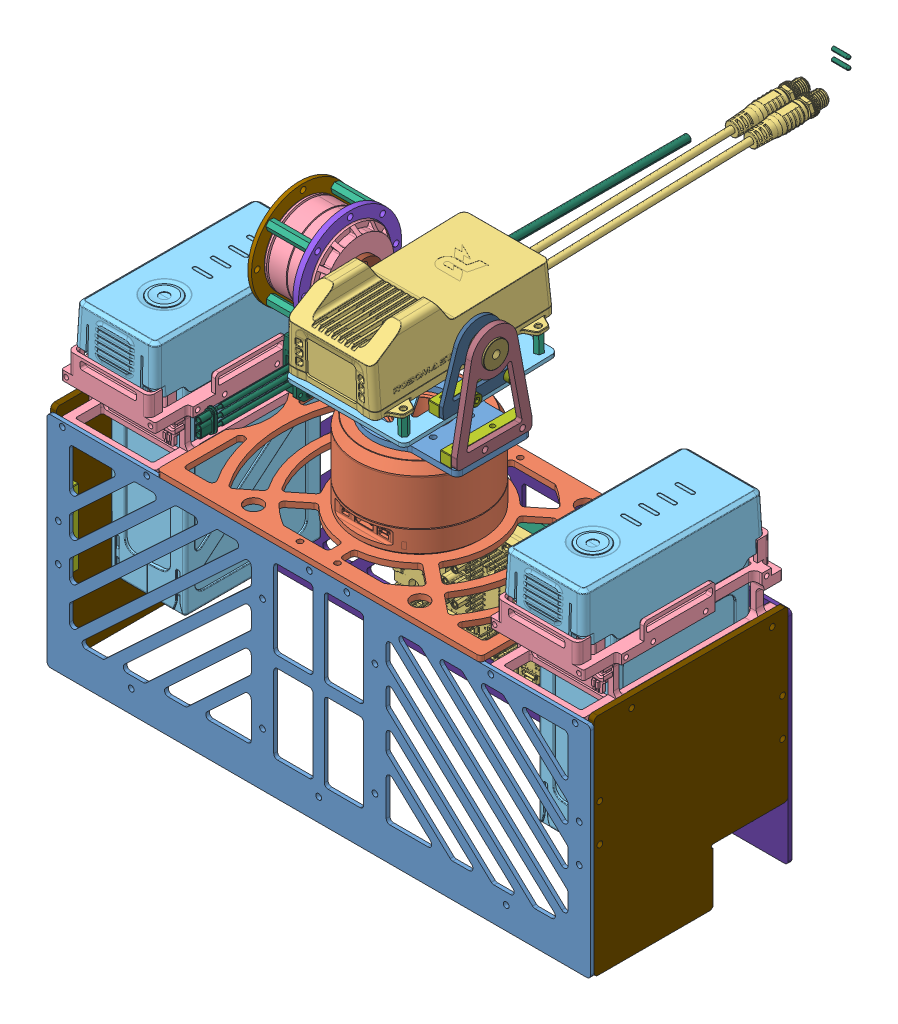
SolidWorks assembly 器件模块总装1.0, configuration 默认. Lengths in mm.
Overall size (300.9 248.89 343.45).
49 component instances, 25 part files, 45 mates.
Components (placement in the parent):
- 图传云台模块-1: 图传云台模块 [默认] at origin size (115.96 130.39 343.45) (flexible)
  - 6020电机传动板-1: 6020电机传动板 [默认] x (1 0 0) z (0 -1 0) size (80 50 3)
  - RoboMaster GM6020 直流无刷电机-1: RoboMaster GM6020 直流无刷电机 [默认] at (0 72.0479 0) x (-0.5 0 -0.866025) z (0 1 0) size (66.7 66.7 45)
  - RoboMaster 图传模块 VT02 2019-1: RoboMaster 图传模块 VT02 2019 [默认] at (0 34.005 -0.333) x (-1 0 0) z (0 0.03027 -0.999542) size (60 36.29 258.03)
  - RoboMaster M3508直流无刷电机转子-1: RoboMaster M3508直流无刷电机转子 [默认] at (-11.659 32.3995 -13.3475) x (0 -0.790596 0.612338) z (-1 0 0) size (42 42 43.4)
  - 图传安装板-1: 图传安装板 [默认] at (0 20.0115 -0.7568) x (1 0 0) z (0 -0.999542 -0.03027) size (64 82 2)
  - 304不锈钢柱-1: 304不锈钢柱 [M2*10] at (27 23.9194 35.3781) x (-0.601616 -0.02418 0.798419) z (0 -0.999542 -0.03027) size (4.62 4 10)
  - 304不锈钢柱-2: 304不锈钢柱 [M2*10] at (-27 23.9194 35.3781) x (-0.601616 -0.02418 0.798419) z (0 -0.999542 -0.03027) size (4.62 4 10)
  - 304不锈钢柱-3: 304不锈钢柱 [M2*10] at (27 26.0989 -36.5889) x (-0.956324 -0.008848 0.292175) z (0 -0.999542 -0.03027) size (4.62 4 10)
  - 304不锈钢柱-4: 304不锈钢柱 [M2*10] at (-27 26.0989 -36.5889) x (0.570383 -0.024864 0.821002) z (0 -0.999542 -0.03027) size (4.62 4 10)
  - 四孔直角转接件-1: 四孔直角转接件 [上交角件] at (-26 23.0101 -0.666) x (1 0 0) z (0 -0.03027 0.999542) size (6 6 40)
  - 四孔直角转接件-2: 四孔直角转接件 [上交角件] at (27 23.0101 -0.666) x (1 0 0) z (0 -0.03027 0.999542) size (6 6 40)
  - 云台转接板-1: 云台转接板 [默认] at (-37 45 0) x (0 0 1) z (-1 0 0) size (55 72.5 3.26)
  - 3508定子安装板-1: 3508定子安装板 [默认] at (-64.1 45 0) x (0 0.707107 -0.707107) z (1 0 0) size (55 55 2)
  - 云台旋转板-1: 云台旋转板 [默认] at (32 45 0) x (0 -0.03027 0.999542) z (-1 0 0) size (40 37.5 2)
  - 3508传动板-1: 3508传动板 [默认] at (-32 45 0) x (0 0.03027 -0.999542) z (1 0 0) size (40 34.5 3)
  - 法兰轴承-1: 法兰轴承 [4*12*4-1] at (41 45 0) x (0 0.036514 0.999333) z (0 -0.999333 0.036514) size (13.5 4 13.5)
  - 转接板2-1: 转接板2 [默认] at (37 45 0) x (0 0 -1) z (1 0 0) size (40 57.5 3)
  - 推力球轴承-1: 推力球轴承 [F4-9M 4*9*4] at (37 45 0) x (0 0.757396 -0.652956) z (0 0.652956 0.757396) size (9 4 9)
  - 法兰轴承-2: 法兰轴承 [4*12*4-1] at (29 45 0) x (0 -0.234612 -0.972089) z (0 -0.972089 0.234612) size (13.5 4 13.5)
  - 304不锈钢柱-5: 304不锈钢柱 [M3*22] at (-51 27.6759 17.3241) x (0 -0.514688 -0.857378) z (1 0 0) size (5.43 4.7 22)
  - 304不锈钢柱-6: 304不锈钢柱 [M3*22] at (-51 27.6759 -17.3241) x (0 -0.372237 -0.928138) z (1 0 0) size (5.43 4.7 22)
  - 304不锈钢柱-7: 304不锈钢柱 [M3*22] at (-51 62.3241 -17.3241) x (0 -0.251026 -0.96798) z (1 0 0) size (5.43 4.7 22)
  - 304不锈钢柱-8: 304不锈钢柱 [M3*22] at (-51 62.3241 17.3241) x (0 -0.159705 -0.987165) z (1 0 0) size (5.43 4.7 22)
  - 四孔直角转接件-3: 四孔直角转接件 [上交角件] at (34 3 0) size (6 6 40)
  - 四孔直角转接件-4: 四孔直角转接件 [上交角件] at (-34 3 0) size (6 6 40)
  - C620无刷电机调速器-1: C620无刷电机调速器 [默认] at (-45.4 6.2704 2.5313) x (0 0 1) z (0 1 0) size (343.45 13.81 26.13)
  - 12.9级圆柱头螺钉-1: 12.9级圆柱头螺钉 [M3*8] at (35 22.8587 4.3318) x (0 -0.455873 -0.890045) z (1 0 0) size (5.68 5.68 11)
  - 12.9级圆柱头螺钉-2: 12.9级圆柱头螺钉 [M3*8] at (35 23.4641 -15.6591) x (0 -0.455873 -0.890045) z (1 0 0) size (5.68 5.68 11)
- 上层器件安装背板-1: 上层器件安装背板 [默认] at (0 -106.5 -52.75) size (290 117 2)
- 元器件安装侧板-1: 元器件安装侧板 [默认] at (143.5 -90 0) x (0 0 -1) z (1 0 0) size (103.5 120 3)
- 元器件安装侧板-2: 元器件安装侧板 [默认] at (-143.5 -90 0) x (0 0 -1) z (1 0 0) size (103.5 120 3)
- 元器件安装前板-1: 元器件安装前板 [默认] at (0 -106.5 52.75) size (290 117 2)
- 元器件安装上板-1: 元器件安装上板 [默认] at (0 -46.5 0) x (-1 0 0) z (0 1 0) size (173 107.5 3)
- 开发板A型-1: 开发板A型 [默认] at (-195.9 -96.5 -343.1489) x (0 -1 0) z (0 0 -1) size (58.4 85.42 16.4)
- 电池装配体-1: 电池装配体 [默认] at (-17.7524 -28.2099 12.1891) x (0 0 1) z (-1 0 0) size (103.5 134.81 69.3)
  - RoboMaster 电池架（兼容型）-1: RoboMaster 电池架（兼容型） [Default] at (-57.9391 2.2099 96.5476) size (103.5 37.5 69.3)
  - TB47S电池-1: TB47S电池 [默认] at (-59.0391 2.7599 97.3476) size (101.5 134.81 44.3)
- 电池装配体-2: 电池装配体 [默认] at (210.8476 -28.2099 12.1891) x (0 0 1) z (-1 0 0) size (103.5 134.81 69.3)
  - RoboMaster 电池架（兼容型）-1: RoboMaster 电池架（兼容型） [Default] at (-57.9391 2.2099 96.5476) size (103.5 37.5 69.3)
  - TB47S电池-1: TB47S电池 [默认] at (-59.0391 2.7599 97.3476) size (101.5 134.81 44.3)
- 四孔直角转接件-1: 四孔直角转接件 [上交角件] at (-139 -100 48.75) x (1 0 0) z (0 -1 0) size (6 6 40)
- 四孔直角转接件-2: 四孔直角转接件 [上交角件] at (-139 -100 -48.75) x (1 0 0) z (0 -1 0) size (6 6 40)
- 四孔直角转接件-3: 四孔直角转接件 [上交角件] at (0 -51 48.75) x (0 1 0) z (1 0 0) size (6 6 40)
- a板安装板-1: a板安装板 [默认] at (0 -97 -41.75) x (0 -1 0) z (-1 0 0) size (72 2 99)
- 304不锈钢接线柱-1: 304不锈钢接线柱 [M3*10-6] at (-46.5 -130 -46.75) size (6 6 10)
- 304不锈钢接线柱-2: 304不锈钢接线柱 [M3*10-6] at (-46.5 -64 -46.75) x (0.999692 0.02482 0) z (0 0 1) size (6 6 10)
- 304不锈钢接线柱-3: 304不锈钢接线柱 [M3*10-6] at (46.5 -130 -46.75) x (0.988734 0.149683 0) z (0 0 1) size (6 6 10)
- 304不锈钢接线柱-4: 304不锈钢接线柱 [M3*10-6] at (46.5 -64 -46.75) x (0.988734 0.149683 0) z (0 0 1) size (6 6 10)
Mates (geometry in assembly coordinates):
- 平行1: parallel anti-aligned: plane of 上层器件安装背板-1 through (0 -106.5 -53.75) normal (0 0 -1)
- 重合2: coincident aligned: plane of 上层器件安装背板-1 through (145 -165 -51.75) normal (1 0 0); plane of 元器件安装侧板-1 through (145 -90 0) normal (1 0 0)
- 重合3: coincident anti-aligned: plane of 上层器件安装背板-1 through (0 -106.5 -51.75) normal (0 0 1); plane of 元器件安装侧板-1 through (145 -135 -51.75) normal (0 0 -1)
- 重合4: coincident aligned: plane of 上层器件安装背板-1 through (145 -165 -51.75) normal (1 0 0); plane of 元器件安装侧板-1 through (145 -90 0) normal (1 0 0)
- 距离1: distance = 3 mm aligned: plane of 元器件安装侧板-1 through (145 -45 51.75) normal (0 1 0); plane of 上层器件安装背板-1 through (-145 -48 -51.75) normal (0 1 0)
- 重合5: coincident anti-aligned: plane of 图传云台模块-1/RoboMaster GM6020 直流无刷电机-1 through (0 -45 0) normal (0 -1 0); plane of 元器件安装侧板-1 through (145 -45 51.75) normal (0 1 0)
- 重合8: coincident aligned: plane of 元器件安装侧板-1 through (145 -45 51.75) normal (0 1 0); plane of 元器件安装侧板-2 through (-142 -45 51.75) normal (0 1 0)
- 重合11: coincident aligned: plane of 上层器件安装背板-1 through (-145 -48 -51.75) normal (0 1 0); plane of 元器件安装前板-1 through (-145 -48 53.75) normal (0 1 0)
- 宽度1: width: plane of 元器件安装前板-1 through (0 -106.5 53.75) normal (0 0 1); plane of 上层器件安装背板-1 through (0 -106.5 -53.75) normal (0 0 -1); cylinder of 图传云台模块-1/RoboMaster GM6020 直流无刷电机-1 through (0 -30.9 0) axis (0 1 0) radius 33.35
- 重合12: coincident anti-aligned: plane of 元器件安装上板-1 through (0 -46.5 0) normal (-1 0 0)
- 重合13: coincident anti-aligned: plane of 元器件安装前板-1 through (-145 -48 53.75) normal (0 1 0); plane of 元器件安装上板-1 through (0 -48 0) normal (0 -1 0)
- 重合14: coincident aligned: plane of 上层器件安装背板-1 through (0 -106.5 -52.75) normal (1 0 0)
- 重合15: coincident anti-aligned: plane of 元器件安装侧板-1 through (145 -135 51.75) normal (0 0 1); plane of 元器件安装前板-1 through (0 -106.5 51.75) normal (0 0 -1)
- 重合16: coincident aligned: plane of 上层器件安装背板-1 through (-145 -165 -51.75) normal (-1 0 0); plane of 元器件安装侧板-2 through (-145 -90 0) normal (-1 0 0)
- 重合17: coincident anti-aligned: plane of 上层器件安装背板-1 through (0 -106.5 -51.75) normal (0 0 1); plane of 元器件安装侧板-2 through (-142 -135 -51.75) normal (0 0 -1)
- 重合20: coincident anti-aligned: plane of 元器件安装前板-1 through (0 -106.5 51.75) normal (0 0 -1); plane of 电池装配体-1/RoboMaster 电池架（兼容型）-1 through (-92.55 -73.483 51.75) normal (0 0 1)
- 重合22: coincident aligned: plane of 元器件安装前板-1 through (-145 -48 53.75) normal (0 1 0); plane of 电池装配体-1/RoboMaster 电池架（兼容型）-1 through (-149.0711 -48 34.25) normal (0 1 0)
- 重合23: coincident anti-aligned: plane of 元器件安装侧板-2 through (-142 -90 0) normal (1 0 0); plane of 电池装配体-1/RoboMaster 电池架（兼容型）-1 through (-142 -53.0001 42.4494) normal (-1 0 0)
- 重合24: coincident anti-aligned: plane of 元器件安装侧板-1 through (142 -90 0) normal (-1 0 0); plane of 电池装配体-2/RoboMaster 电池架（兼容型）-1 through (142 -53.0001 -55.62) normal (1 0 0)
- 重合25: coincident anti-aligned: plane of 元器件安装前板-1 through (0 -106.5 51.75) normal (0 0 -1); plane of 电池装配体-2/RoboMaster 电池架（兼容型）-1 through (136.05 -73.483 51.75) normal (0 0 1)
- 重合26: coincident aligned: plane of 元器件安装前板-1 through (-145 -48 53.75) normal (0 1 0); plane of 电池装配体-2/RoboMaster 电池架（兼容型）-1 through (79.5289 -48 34.25) normal (0 1 0)
- 距离2: distance = 12 mm anti-aligned: plane of 开发板A型-1 through (0 -97 -39.75) normal (0 0 -1); plane of 上层器件安装背板-1 through (0 -106.5 -51.75) normal (0 0 1)
- 距离3: distance = 20 mm aligned: plane of 开发板A型-1 through (-42.5 -68 -32.75) normal (0 1 0); plane of 上层器件安装背板-1 through (-145 -48 -51.75) normal (0 1 0)
- 同心1: concentric anti-aligned: cylinder of 图传云台模块-1/RoboMaster GM6020 直流无刷电机-1 through (-25.1147 -36.1088 14.5) axis (0 -1 0) radius 1.8; cylinder of 元器件安装上板-1 through (-25.1147 -55 14.5) axis (0 1 0) radius 2.025
- 重合27: coincident anti-aligned: plane of 元器件安装前板-1 through (0 -106.5 51.75) normal (0 0 -1); plane of 四孔直角转接件-1 through (-142 -120 51.75) normal (0 0 1)
- 重合28: coincident anti-aligned: plane of 元器件安装侧板-2 through (-142 -90 0) normal (1 0 0); plane of 四孔直角转接件-1 through (-142 -120 45.75) normal (-1 0 0)
- 距离5: distance = 45 mm aligned: plane of 四孔直角转接件-1 through (-139 -120 48.75) normal (0 -1 0); plane of 元器件安装侧板-2 through (-215.23 -165 51.75) normal (0 -1 0)
- 重合29: coincident anti-aligned: plane of 上层器件安装背板-1 through (0 -106.5 -51.75) normal (0 0 1); plane of 四孔直角转接件-2 through (-142 -120 -51.75) normal (0 0 -1)
- 重合30: coincident anti-aligned: plane of 元器件安装侧板-2 through (-142 -90 0) normal (1 0 0); plane of 四孔直角转接件-2 through (-142 -120 -51.75) normal (-1 0 0)
- 重合31: coincident aligned: plane of 四孔直角转接件-1 through (-139 -120 48.75) normal (0 -1 0); plane of 四孔直角转接件-2 through (-139 -120 -48.75) normal (0 -1 0)
- 重合32: coincident anti-aligned: plane of 元器件安装上板-1 through (0 -48 0) normal (0 -1 0); plane of 四孔直角转接件-3 through (20 -48 45.75) normal (0 1 0)
- 重合33: coincident anti-aligned: plane of 元器件安装前板-1 through (0 -106.5 51.75) normal (0 0 -1); plane of 四孔直角转接件-3 through (20 -54 51.75) normal (0 0 1)
- 宽度2: width anti-aligned: plane of 元器件安装上板-1 through (86.5 -55 53.75) normal (1 0 0); plane of 元器件安装上板-1 through (-86.5 -55 53.75) normal (-1 0 0); plane of 四孔直角转接件-3 through (-20 -51 48.75) normal (-1 0 0); plane of 四孔直角转接件-3 through (20 -51 48.75) normal (1 0 0)
- 宽度3: width anti-aligned: plane of 元器件安装侧板-2 through (-142 -90 0) normal (1 0 0); plane of 开发板A型-1 through (142 -90 0) normal (-1 0 0); plane of 元器件安装侧板-1 through (-42.5 -68 -149.6529) normal (-1 0 0); plane of 开发板A型-1 through (42.5 -68 -149.6529) normal (1 0 0)
- 重合34: coincident anti-aligned: plane of 开发板A型-1 through (0 -97 -39.75) normal (0 0 -1); plane of a板安装板-1 through (0 -97 -39.75) normal (0 0 1)
- 同心2: concentric aligned: cylinder of 开发板A型-1 through (-32 -113 -149.6529) axis (0 0 1) radius 1.75; cylinder of a板安装板-1 through (-32 -113 -41.75) axis (0 0 1) radius 1.525
- 同心3: concentric aligned: cylinder of 开发板A型-1 through (32 -81 -149.6529) axis (0 0 1) radius 1.75; cylinder of a板安装板-1 through (32 -81 -41.75) axis (0 0 1) radius 1.525
- 同心4: concentric aligned: cylinder of a板安装板-1 through (-46.5 -130 -41.75) axis (0 0 1) radius 1.525; cylinder of 304不锈钢接线柱-1 through (-46.5 -130 -41.75) axis (0 0 1) radius 3
- 重合35: coincident anti-aligned: plane of a板安装板-1 through (0 -97 -41.75) normal (0 0 -1); plane of 304不锈钢接线柱-1 through (-46.5 -127 -41.75) normal (0 0 1)
- 同心5: concentric aligned: cylinder of a板安装板-1 through (-46.5 -64 -41.75) axis (0 0 1) radius 1.525; cylinder of 304不锈钢接线柱-2 through (-46.5 -64 -41.75) axis (0 0 1) radius 3
- 重合36: coincident anti-aligned: plane of a板安装板-1 through (0 -97 -41.75) normal (0 0 -1); plane of 304不锈钢接线柱-2 through (-46.5745 -61.0009 -41.75) normal (0 0 1)
- 同心6: concentric aligned: cylinder of a板安装板-1 through (46.5 -130 -41.75) axis (0 0 1) radius 1.525; cylinder of 304不锈钢接线柱-3 through (46.5 -130 -41.75) axis (0 0 1) radius 3
- 重合37: coincident anti-aligned: plane of a板安装板-1 through (0 -97 -41.75) normal (0 0 -1); plane of 304不锈钢接线柱-3 through (46.051 -127.0338 -41.75) normal (0 0 1)
- 同心7: concentric aligned: cylinder of a板安装板-1 through (46.5 -64 -41.75) axis (0 0 1) radius 1.525; cylinder of 304不锈钢接线柱-4 through (46.5 -64 -41.75) axis (0 0 1) radius 3
- 重合38: coincident anti-aligned: plane of a板安装板-1 through (0 -97 -41.75) normal (0 0 -1); plane of 304不锈钢接线柱-4 through (46.051 -61.0338 -41.75) normal (0 0 1)
